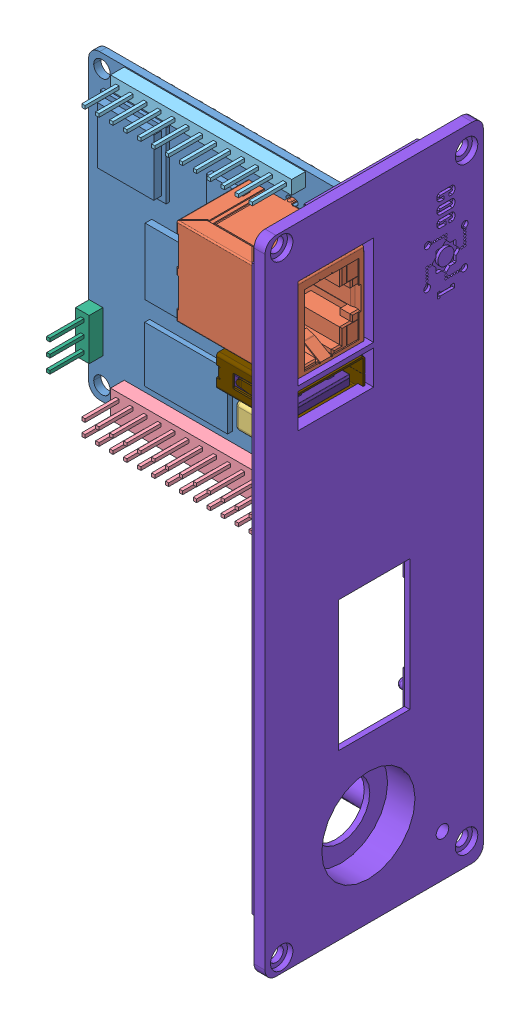
SolidWorks assembly front_assembly, configuration Default. Lengths in mm.
Overall size (52 117 39.8).
31 component instances, 26 part files, 3 mates.
Components (placement in the parent):
- pcb-assy_asm.stp-1: pcb-assy_asm.stp [Default] at origin size (50.95 55 17.13)
  - JYS-TF130-021_ASM.stp-1: JYS-TF130-021_ASM.stp [Default] at (-24 15.75 -2.7) x (0 -1 0) z (1 0 0) size (11.53 1.3 11.26)
    - MSBR-10.stp-1: MSBR-10.stp [Default] at origin size (11.53 1.3 9.25)
    - MSBR-9.stp-1: MSBR-9.stp [Default] at origin size (0.62 0.94 9.2)
    - MSBR-8.stp-1: MSBR-8.stp [Default] at origin size (0.76 1.05 6.18)
    - MSBR-7.stp-1: MSBR-7.stp [Default] at origin size (0.75 1 6.15)
    - MSBR-6.stp-1: MSBR-6.stp [Default] at origin size (0.75 1.05 6.48)
    - MSBR-5.stp-1: MSBR-5.stp [Default] at origin size (0.75 1.05 6.48)
    - MSBR-4.stp-1: MSBR-4.stp [Default] at origin size (0.75 1.05 6.48)
    - MSBR-3.stp-1: MSBR-3.stp [Default] at origin size (0.75 1.05 6.48)
    - MSBR-2.stp-1: MSBR-2.stp [Default] at origin size (0.75 1.05 6.48)
    - MSBR-1.stp-1: MSBR-1.stp [Default] at origin size (0.76 1.05 6.73)
    - _JYS-TF130-021.stp-1: _JYS-TF130-021.stp [Default] at origin size (11.51 1.3 11.26)
  - _USB_ASM_3_ASM.stp-1: _USB_ASM_3_ASM.stp [Default] at (6.79 1.5 7.2) x (0 0 -1) z (1 0 0) size (17.04 5.71 13.86)
    - PIN1_ASM_3_ASM.stp-1: PIN1_ASM_3_ASM.stp [Default] at origin size (14.51 4.86 6.54)
      - PIN1_1_3.stp-1: PIN1_1_3.stp [Default] at origin size (7.31 2.84 6.53)
      - PIN1_2_3.stp-1: PIN1_2_3.stp [Default] at origin size (9.81 1.86 6.53)
      - PIN1_3_3.stp-1: PIN1_3_3.stp [Default] at origin size (12.01 2.58 6.54)
      - PIN1_4_3.stp-1: PIN1_4_3.stp [Default] at origin size (14.51 3.88 6.53)
    - _X2_585180F6_X0_1_3_ASM.stp-1: _X2_585180F6_X0_1_3_ASM.stp [Default] at (0 0 0.9) size (13.45 5.6 12.5)
      - _X2_585180F6_X0_1_3_1.stp-1: _X2_585180F6_X0_1_3_1.stp [Default] at origin size (13.45 5.6 7)
      - _X2_585180F6_X0_1_3_2.stp-1: _X2_585180F6_X0_1_3_2.stp [Default] at origin size (10.6 1.81 11.3)
    - _X2_76F48FB991D15C5E58F3_X0__4.stp-1: _X2_76F48FB991D15C5E58F3_X0__4.stp [Default] at origin size (13.75 5.71 13.86)
  - PCB-Z3.stp-1: PCB-Z3.stp [Default] at origin size (50 55 5.3)
  - RJ45.stp-1: RJ45.stp [Default] at (25.5837 13.6737 0.9116) x (0 -1 0) z (1 0 0) size (16.44 17.12 21.1)
  - TYPE_C_CC.stp-1: TYPE_C_CC.stp [Default] at (21.1704 -7.7205 5.11) x (0 0 -1) z (0 -1 0) size (11.43 14.3 4.52)
  - 26PIN_CONN.stp-1: 26PIN_CONN.stp [Default] at (-3.2711 -24.6266 0) size (33.02 5 11.2)
  - 13PIN-CONN-SIMPLE.stp-1: 13PIN-CONN-SIMPLE.stp [Default] at (-0.7211 27.3126 0) x (-1 0 0) z (0 0 1) size (33.02 2.5 11.2)
  - 3PIN-CONN-SIMPLE.stp-1: 3PIN-CONN-SIMPLE.stp [Default] at (-22.3935 -17.6899 0) x (0 1 0) z (0 0 1) size (7.62 2.5 11.2)
  - 03_11_13_0003_HDMI0001.stp-1: 03_11_13_0003_HDMI0001.stp [Default] at (25.92 -18.43 1.63) x (0 1 0) z (0 0 -1) size (8.9 7.5 3.76)
- cog-1-front-lid-1: cog-1-front-lid [Default] at (25 -26.0766 -0.05) x (0 1 0) z (0 0 -1) size (117 18 39.8)
Mates (geometry in assembly coordinates):
- Coincident1: coincident anti-aligned: plane of pcb-assy_asm.stp-1/PCB-Z3.stp-1 through (25 -27.5 0) normal (1 0 0); plane of cog-1-front-lid-1 through (25 30.4234 17.85) normal (-1 0 0)
- Distance5: distance = 11 mm: line of cog-1-front-lid-1 through (25 -83.5766 11) axis (0 1 0); line of pcb-assy_asm.stp-1/PCB-Z3.stp-1 through (51 25 -25.5) axis (0 0 1)
- Distance6: distance = 57.4 mm: plane of pcb-assy_asm.stp-1/26PIN_CONN.stp-1 through (12.9439 -26.1766 10) normal (0 -1 0); line of cog-1-front-lid-1 through (25 -83.5766 11) axis (0 0 1)
